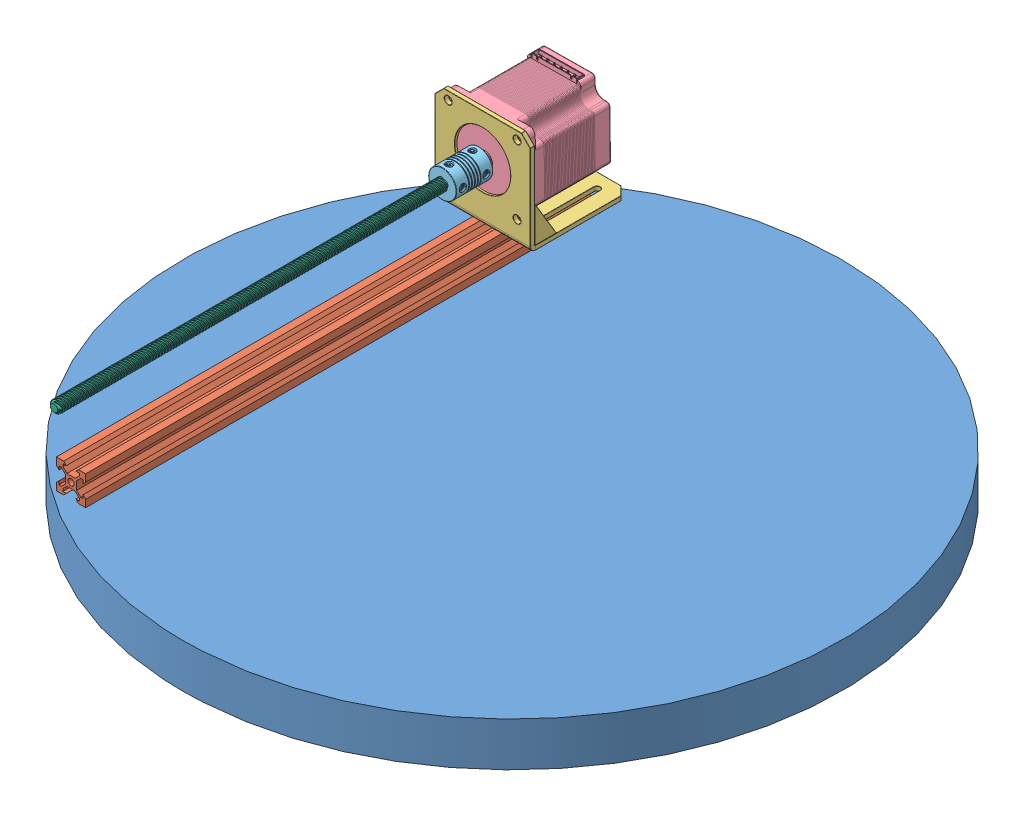
SolidWorks assembly MainAssembly, configuration Predeterminado. Lengths in mm.
Overall size (450 120.18 450).
7 component instances, 6 part files, 1 mates.
Components (placement in the parent):
- Base-1: Base [Predeterminado] at (-15.8252 -39.2033 450) size (450 30 450)
- AxisX1-1: AxisX1 [Predeterminado] at (-131.8499 1.1715 104.6648) size (65 90.18 362.48)
  - BoschAxisX-1: BoschAxisX [Predeterminado] at (-15.3809 9.6252 175) size (20 20 350)
  - BracketNEMA23-1: BracketNEMA23 [Default] at (-6.5235 12.6252 243) x (0 0 -1) z (1 0 0) size (68 68 65)
  - Nema 23-1: Nema 23 [Default] at (-6.3512 48.3154 184) x (0.999948 0.010225 0) z (0 0 1) size (56.4 59.4 76.6)
  - Coupler 6.35-8mm-1: Coupler 6.35-8mm [Default] at (-6.3512 48.3154 258.1) size (19.34 19.34 25)
  - ScrewAxisX-2: ScrewAxisX [Default] at (-6.3512 48.3154 135.6) x (-0.923728 -0.383049 0) z (0 0 -1) size (8.33 8.33 279.26)
Mates (geometry in assembly coordinates):
- Coincidente1: coincident anti-aligned: plane of Base-1 through (-15.8252 -9.2033 450) normal (0 1 0); plane of AxisX1-1/BoschAxisX-1 through (-147.2308 -9.2033 629.6648) normal (0 -1 0)
